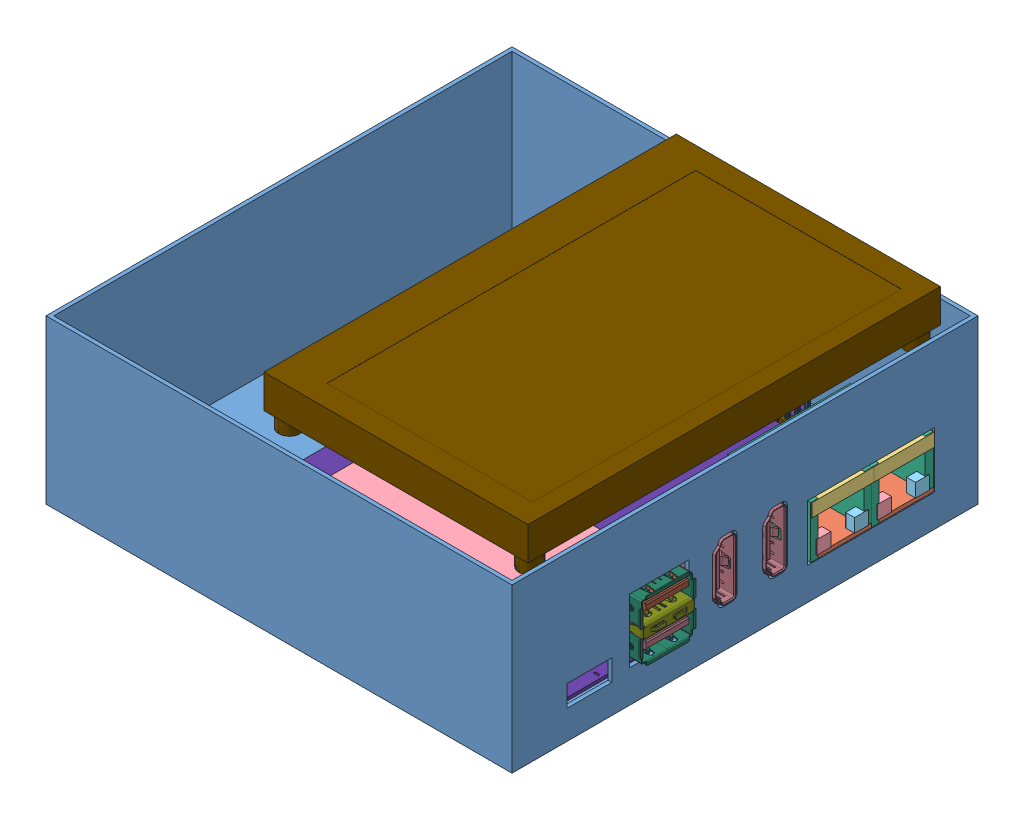
SolidWorks assembly bilbo-hub, configuration Default. Lengths in mm. (continued)
Components (placement in the parent): (continued)
- CM4-DUAL-ETH-4G 5G-BASE-1: CM4-DUAL-ETH-4G 5G-BASE [Default] at (-27.9996 8.7984 -51.6437) x (1 0 0.000117) z (0 1 0) size (91.94 99.62 20.53) (continued)
  - CM4-DUAL-ETH-4G 5G-BASE.step-1: CM4-DUAL-ETH-4G 5G-BASE.step [Default] at origin size (91.94 99.62 20.53) (continued)
    - C49.step-1: C49.step [Default] at origin size (0.8 1.6 0.6) (continued)
      - CAPC1608(0603).step-1: CAPC1608(0603).step [Default] at (38.0407 -61.99 0) x (0 -1 0) z (0 0 1) size (1.6 0.8 0.6)
    - C48.step-1: C48.step [Default] at origin size (1.6 0.8 0.6)
      - CAPC1608(0603).step-1: CAPC1608(0603).step [Default] at (49.0658 -69.8064 0) x (-1 0 0) z (0 0 1) size (1.6 0.8 0.6)
    - C47.step-1: C47.step [Default] at origin size (0.8 1.6 0.6)
      - CAPC1608(0603).step-1: CAPC1608(0603).step [Default] at (39.4963 -61.99 0) x (0 -1 0) z (0 0 1) size (1.6 0.8 0.6)
    - C46.step-1: C46.step [Default] at origin size (1.6 0.8 0.6)
      - CAPC1608(0603).step-1: CAPC1608(0603).step [Default] at (49.0658 -71.2537 0) x (-1 0 0) z (0 0 1) size (1.6 0.8 0.6)
    - C44.step-1: C44.step [Default] at origin size (0.8 1.6 0.6)
      - CAPC1608(0603).step-1: CAPC1608(0603).step [Default] at (42.5195 -81.9688 -0.7984) x (0 1 0) z (0 0 -1) size (1.6 0.8 0.6)
    - C43.step-1: C43.step [Default] at origin size (1.6 0.8 0.6)
      - CAPC1608(0603).step-1: CAPC1608(0603).step [Default] at (49.1866 -62.69 0) x (-1 0 0) z (0 0 1) size (1.6 0.8 0.6)
    - C42.step-1: C42.step [Default] at origin size (1.6 0.8 0.6)
      - CAPC1608(0603).step-1: CAPC1608(0603).step [Default] at (49.0658 -74.1482 0) x (-1 0 0) z (0 0 1) size (1.6 0.8 0.6)
    - C41.step-1: C41.step [Default] at origin size (0.8 1.6 0.6)
      - CAPC1608(0603).step-1: CAPC1608(0603).step [Default] at (52.2225 -27.9219 -0.7984) x (0 1 0) z (0 0 -1) size (1.6 0.8 0.6)
    - C40.step-1: C40.step [Default] at origin size (1.6 0.8 0.6)
      - CAPC1608(0603).step-1: CAPC1608(0603).step [Default] at (49.1866 -63.8607 0) x (-1 0 0) z (0 0 1) size (1.6 0.8 0.6)
    - C39.step-1: C39.step [Default] at origin size (1.6 0.8 0.6)
      - CAPC1608(0603).step-1: CAPC1608(0603).step [Default] at (48.9722 -75.5798 0) x (-1 0 0) z (0 0 1) size (1.6 0.8 0.6)
    - C32.step-1: C32.step [Default] at origin size (1.6 0.8 0.6)
      - CAPC1608(0603).step-1: CAPC1608(0603).step [Default] at (51.5062 -32.7167 -0.7984) x (-1 0 0) z (0 0 -1) size (1.6 0.8 0.6)
    - C31.step-1: C31.step [Default] at origin size (0.8 1.6 0.6)
      - CAPC1608(0603).step-1: CAPC1608(0603).step [Default] at (48.8898 -27.9219 -0.7984) x (0 1 0) z (0 0 -1) size (1.6 0.8 0.6)
    - C30.step-1: C30.step [Default] at origin size (0.8 1.6 0.6)
      - CAPC1608(0603).step-1: CAPC1608(0603).step [Default] at (50.6641 -41.4202 -0.7984) x (0 1 0) z (0 0 -1) size (1.6 0.8 0.6)
    - C28.step-1: C28.step [Default] at origin size (0.8 1.6 0.6)
      - CAPC1608(0603).step-1: CAPC1608(0603).step [Default] at (53.758 -41.4202 -0.7984) x (0 1 0) z (0 0 -1) size (1.6 0.8 0.6)
    - C27.step-1: C27.step [Default] at origin size (0.8 1.6 0.6)
      - CAPC1608(0603).step-1: CAPC1608(0603).step [Default] at (52.2222 -41.4202 -0.7984) x (0 1 0) z (0 0 -1) size (1.6 0.8 0.6)
    - C26.step-1: C26.step [Default] at origin size (1.6 0.8 0.6)
      - CAPC1608(0603).step-1: CAPC1608(0603).step [Default] at (51.5325 -31.2588 -0.7984) x (1 0 0) z (0 0 -1) size (1.6 0.8 0.6)
    - C22.step-1: C22.step [Default] at origin size (1.6 0.8 0.6)
      - CAPC1608(0603).step-1: CAPC1608(0603).step [Default] at (51.5318 -35.5502 -0.7984) x (1 0 0) z (0 0 -1) size (1.6 0.8 0.6)
    - C21.step-1: C21.step [Default] at origin size (1.6 0.8 0.6)
      - CAPC1608(0603).step-1: CAPC1608(0603).step [Default] at (51.5318 -38.3867 -0.7984) x (1 0 0) z (0 0 -1) size (1.6 0.8 0.6)
    - C4.step-1: C4.step [Default] at origin size (0.8 1.6 0.6)
      - CAPC1608(0603).step-1: CAPC1608(0603).step [Default] at (56.9561 -77.7112 -0.7984) x (0 -1 0) z (0 0 -1) size (1.6 0.8 0.6)
    - C3.step-1: C3.step [Default] at origin size (1.27 2.72 0.46)
      - 663598576.step-1: 663598576.step [Default] at (56.9823 -82.7935 -1.2584) size (1.27 0.28 0.46)
        - Extruded-45.step-1: Extruded-45.step [Default] at origin size (1.27 0.28 0.46)
      - 663598576.step-2: 663598576.step [Default] at (56.9823 -80.3446 -1.2584) size (1.27 0.28 0.46)
        - Extruded-45.step-1: Extruded-45.step [Default] at origin size (1.27 0.28 0.46)
      - 764368928.step-1: 764368928.step [Default] at (56.9823 -81.6251 -1.2484) size (1.12 2.29 0.42)
        - Extruded-46.step-1: Extruded-46.step [Default] at origin size (1.12 2.29 0.42)
    - AMS-1.step-1: AMS-1.step [Default] at origin size (6.73 3.43 1.02)
      - 880594240.step-1: 880594240.step [Default] at (36.1772 -86.6648 0.254) size (6.73 3.43 1.02)
        - Extruded-47.step-1: Extruded-47.step [Default] at origin size (6.73 3.43 1.02)
    - R11.step-1: R11.step [Default] at origin size (0.8 1.6 0.38)
      - RESC1608(0603).step-1: RESC1608(0603).step [Default] at (64.5833 -30.5497 -0.7984) x (0 -1 0) z (1 0 0) size (1.6 0.38 0.8)
    - U3.step-1: U3.step [Default] at origin size (7.8 5.3 2.16)
      - 1503579216.step-1: 1503579216.step [Default] at (33.3767 -82.4828 -1.0524) size (1.3 0.41 0.25)
        - Extruded-48.step-1: Extruded-48.step [Default] at origin size (1.3 0.41 0.25)
      - 1503579216.step-2: 1503579216.step [Default] at (33.3767 -81.2128 -1.0524) size (1.3 0.41 0.25)
        - Extruded-48.step-1: Extruded-48.step [Default] at origin size (1.3 0.41 0.25)
      - 1503579216.step-3: 1503579216.step [Default] at (33.3767 -79.9428 -1.0524) size (1.3 0.41 0.25)
        - Extruded-48.step-1: Extruded-48.step [Default] at origin size (1.3 0.41 0.25)
      - 1503579216.step-4: 1503579216.step [Default] at (33.3767 -78.6728 -1.0524) size (1.3 0.41 0.25)
        - Extruded-48.step-1: Extruded-48.step [Default] at origin size (1.3 0.41 0.25)
      - 1503579216.step-5: 1503579216.step [Default] at (39.8767 -82.4928 -1.0524) size (1.3 0.41 0.25)
        - Extruded-48.step-1: Extruded-48.step [Default] at origin size (1.3 0.41 0.25)
      - 1503579216.step-6: 1503579216.step [Default] at (39.8767 -81.2228 -1.0524) size (1.3 0.41 0.25)
        - Extruded-48.step-1: Extruded-48.step [Default] at origin size (1.3 0.41 0.25)
      - 1503579216.step-7: 1503579216.step [Default] at (39.8767 -79.9528 -1.0524) size (1.3 0.41 0.25)
        - Extruded-48.step-1: Extruded-48.step [Default] at origin size (1.3 0.41 0.25)
      - 1503579216.step-8: 1503579216.step [Default] at (39.8767 -78.6828 -1.0524) size (1.3 0.41 0.25)
        - Extruded-48.step-1: Extruded-48.step [Default] at origin size (1.3 0.41 0.25)
      - 1503581520.step-1: 1503581520.step [Default] at (36.6267 -80.5828 -2.9584) size (5.4 5.3 2.01)
        - Extruded-49.step-1: Extruded-49.step [Default] at origin size (5.4 5.3 2.01)
    - R18.step-1: R18.step [Default] at origin size (0.8 1.6 0.38)
      - RESC1608(0603).step-1: RESC1608(0603).step [Default] at (36.3808 -80.8002 0) x (0 -1 0) z (-1 0 0) size (1.6 0.38 0.8)
    - R17.step-1: R17.step [Default] at origin size (1.6 0.8 0.38)
      - RESC1608(0603).step-1: RESC1608(0603).step [Default] at (29.8754 -75.3761 0) x (-1 0 0) z (0 1 0) size (1.6 0.38 0.8)
    - R16.step-1: R16.step [Default] at origin size (0.8 1.6 0.38)
      - RESC1608(0603).step-1: RESC1608(0603).step [Default] at (30.3209 -79.2715 -0.7984) x (0 -1 0) z (1 0 0) size (1.6 0.38 0.8)
    - R15.step-1: R15.step [Default] at origin size (0.8 1.6 0.38)
      - RESC1608(0603).step-1: RESC1608(0603).step [Default] at (50.6744 -27.9001 -0.7984) x (0 1 0) z (-1 0 0) size (1.6 0.38 0.8)
    - U4.step-1: U4.step [Default] at origin size (2.7 2.7 0.45)
      - 880596160.step-1: 880596160.step [Default] at (49.7296 -17.227 -1.2984) size (2.7 2.7 0.45)
        - Extruded-50.step-1: Extruded-50.step [Default] at origin size (2.7 2.7 0.45)
    - U5.step-1: U5.step [Default] at origin size (2 2.1 0.95)
      - User_Library-SC70-5-1.step-1: User_Library-SC70-5-1.step [Default] at (52.8539 -17.1936 -0.7984) x (1 0 0) z (0 0 -1) size (2 2.1 0.95)
    - R35.step-1: R35.step [Default] at origin size (0.8 1.6 0.38)
      - RESC1608(0603).step-1: RESC1608(0603).step [Default] at (52.2527 -11.5783 -0.7984) x (0 1 0) z (-1 0 0) size (1.6 0.38 0.8)
    - R33.step-1: R33.step [Default] at origin size (0.8 1.6 0.38)
      - RESC1608(0603).step-1: RESC1608(0603).step [Default] at (53.7884 -11.5783 -0.7984) x (0 1 0) z (-1 0 0) size (1.6 0.38 0.8)
    - D6.step-1: D6.step [Default] at origin size (1.35 2.6 1.14)
      - SW3dPS-SOD-323.step-1: SW3dPS-SOD-323.step [Default] at (51.0946 -21.502 -0.7984) x (0 -1 0) z (0 0 -1) size (2.6 1.35 1.14)
    - D5.step-1: D5.step [Default] at origin size (1.35 2.6 1.14)
      - SW3dPS-SOD-323.step-1: SW3dPS-SOD-323.step [Default] at (53.3476 -21.502 -0.7984) x (0 -1 0) z (0 0 -1) size (2.6 1.35 1.14)
    - C134.step-1: C134.step [Default] at origin size (0.8 1.6 0.6)
      - CAPC1608(0603).step-1: CAPC1608(0603).step [Default] at (55.1652 -21.3602 -0.7984) x (0 1 0) z (0 0 -1) size (1.6 0.8 0.6)
    - C133.step-1: C133.step [Default] at origin size (0.8 1.6 0.6)
      - CAPC1608(0603).step-1: CAPC1608(0603).step [Default] at (49.1745 -21.3865 -0.7984) x (0 -1 0) z (0 0 -1) size (1.6 0.8 0.6)
    - C38.step-1: C38.step [Default] at origin size (1.6 0.8 0.6)
      - CAPC1608(0603).step-1: CAPC1608(0603).step [Default] at (54.6319 -14.1546 -0.7984) x (1 0 0) z (0 0 -1) size (1.6 0.8 0.6)
    - C37.step-1: C37.step [Default] at origin size (0.8 1.6 0.6)
      - CAPC1608(0603).step-1: CAPC1608(0603).step [Default] at (55.1653 -17.2646 -0.7984) x (0 1 0) z (0 0 -1) size (1.6 0.8 0.6)
    - C36.step-1: C36.step [Default] at origin size (0.8 1.6 0.6)
      - CAPC1608(0603).step-1: CAPC1608(0603).step [Default] at (50.7103 -11.6263 -0.7984) x (0 -1 0) z (0 0 -1) size (1.6 0.8 0.6)
    - C35.step-1: C35.step [Default] at origin size (0.8 1.6 0.6)
      - CAPC1608(0603).step-1: CAPC1608(0603).step [Default] at (49.1745 -11.6263 -0.7984) x (0 -1 0) z (0 0 -1) size (1.6 0.8 0.6)
    - C9.step-1: C9.step [Default] at origin size (0.8 1.6 0.6)
      - CAPC1608(0603).step-1: CAPC1608(0603).step [Default] at (17.7596 -11.9503 -0.7984) x (0 1 0) z (0 0 -1) size (1.6 0.8 0.6)
    - C14.step-1: C14.step [Default] at origin size (0.8 1.6 0.6)
      - CAPC1608(0603).step-1: CAPC1608(0603).step [Default] at (77.2667 -94.9453 -0.7984) x (0 -1 0) z (0 0 -1) size (1.6 0.8 0.6)
    - C1.step-1: C1.step [Default] at origin size (0.8 1.6 0.6)
      - CAPC1608(0603).step-1: CAPC1608(0603).step [Default] at (39.7941 -94.4916 -0.7984) x (0 -1 0) z (0 0 -1) size (1.6 0.8 0.6)
    - U15.step-1: U15.step [Default] at origin size (2.5 3 1.1)
      - SW3DPS-SOT-23-5-DEFAULT.step-1: SW3DPS-SOT-23-5-DEFAULT.step [Default] at (9.4742 -18.2293 -1.2984) x (0 1 0) z (-1 0 0) size (3 1.1 2.5)
    - U12.step-1: U12.step [Default] at origin size (1.01 2.5 0.55)
      - User_Library-UDFN10.step-1: User_Library-UDFN10.step [Default] at (62.7073 -10.1236 0.1516) x (0 -1 0) z (1 0 0) size (2.5 0.55 1.01)
        - Body.step-1: Body.step [Default] at (1.0785 0.9721 1.8983) size (2.5 0.5 1)
        - Pin1.step-1: Pin1.step [Default] at (0.0785 1.0521 2.2208) x (0 0 -1) z (-1 0 0) size (0.36 0.13 0.2)
        - Pin2.step-1: Pin2.step [Default] at (0.5785 1.0521 2.2208) x (0 0 1) z (1 0 0) size (0.36 0.13 0.2)
        - Pin4.step-1: Pin4.step [Default] at (1.0785 0.9221 2.2208) x (0 0 1) z (-1 0 0) size (0.49 0.13 0.4)
        - Pin2.step-2: Pin2.step [Default] at (1.5785 0.9221 2.2208) x (0 0 1) z (-1 0 0) size (0.36 0.13 0.2)
        - Pin2.step-3: Pin2.step [Default] at (2.0785 0.9221 2.2208) x (0 0 1) z (-1 0 0) size (0.36 0.13 0.2)
        - Pin2.step-4: Pin2.step [Default] at (2.0785 0.9221 1.5758) x (0 0 -1) z (1 0 0) size (0.36 0.13 0.2)
        - Pin2.step-5: Pin2.step [Default] at (1.5785 0.9221 1.5758) x (0 0 -1) z (1 0 0) size (0.36 0.13 0.2)
        - Pin3.step-1: Pin3.step [Default] at (1.0785 0.9221 1.5758) x (0 0 1) z (-1 0 0) size (0.36 0.13 0.4)
        - Pin2.step-6: Pin2.step [Default] at (0.5785 0.9221 1.5758) x (0 0 -1) z (1 0 0) size (0.36 0.13 0.2)
        - Pin2.step-7: Pin2.step [Default] at (0.0785 0.9221 1.5758) x (0 0 -1) z (1 0 0) size (0.36 0.13 0.2)
    - U11.step-1: U11.step [Default] at origin size (2.5 3 1.1)
      - SW3DPS-SOT-23-5-DEFAULT.step-1: SW3DPS-SOT-23-5-DEFAULT.step [Default] at (50.4006 -45.1237 -1.2984) x (0 -1 0) z (1 0 0) size (3 1.1 2.5)
    - U9.step-1: U9.step [Default] at origin size (1.01 2.5 0.55)
      - User_Library-UDFN10.step-1: User_Library-UDFN10.step [Default] at (66.4724 -18.6329 0.1516) x (0 1 0) z (-1 0 0) size (2.5 0.55 1.01)
        - Body.step-1: Body.step [Default] at (1.0785 0.9721 1.8983) size (2.5 0.5 1)
        - Pin1.step-1: Pin1.step [Default] at (0.0785 1.0521 2.2208) x (0 0 -1) z (-1 0 0) size (0.36 0.13 0.2)
        - Pin2.step-1: Pin2.step [Default] at (0.5785 1.0521 2.2208) x (0 0 1) z (1 0 0) size (0.36 0.13 0.2)
        - Pin4.step-1: Pin4.step [Default] at (1.0785 0.9221 2.2208) x (0 0 1) z (-1 0 0) size (0.49 0.13 0.4)
        - Pin2.step-2: Pin2.step [Default] at (1.5785 0.9221 2.2208) x (0 0 1) z (-1 0 0) size (0.36 0.13 0.2)
        - Pin2.step-3: Pin2.step [Default] at (2.0785 0.9221 2.2208) x (0 0 1) z (-1 0 0) size (0.36 0.13 0.2)
        - Pin2.step-4: Pin2.step [Default] at (2.0785 0.9221 1.5758) x (0 0 -1) z (1 0 0) size (0.36 0.13 0.2)
        - Pin2.step-5: Pin2.step [Default] at (1.5785 0.9221 1.5758) x (0 0 -1) z (1 0 0) size (0.36 0.13 0.2)
        - Pin3.step-1: Pin3.step [Default] at (1.0785 0.9221 1.5758) x (0 0 1) z (-1 0 0) size (0.36 0.13 0.4)
        - Pin2.step-6: Pin2.step [Default] at (0.5785 0.9221 1.5758) x (0 0 -1) z (1 0 0) size (0.36 0.13 0.2)
        - Pin2.step-7: Pin2.step [Default] at (0.0785 0.9221 1.5758) x (0 0 -1) z (1 0 0) size (0.36 0.13 0.2)
    - R64.step-1: R64.step [Default] at origin size (0.8 1.6 0.38)
      - RESC1608(0603).step-1: RESC1608(0603).step [Default] at (12.5285 -18.2821 -0.7984) x (0 -1 0) z (1 0 0) size (1.6 0.38 0.8)
    - R57.step-1: R57.step [Default] at origin size (1.6 0.8 0.38)
      - RESC1608(0603).step-1: RESC1608(0603).step [Default] at (10.7955 -85.6126 0) x (-1 0 0) z (0 1 0) size (1.6 0.38 0.8)
    - R56.step-1: R56.step [Default] at origin size (1.6 0.8 0.38)
      - RESC1608(0603).step-1: RESC1608(0603).step [Default] at (10.8653 -83.8424 0) x (1 0 0) z (0 -1 0) size (1.6 0.38 0.8)
    - R55.step-1: R55.step [Default] at origin size (0.8 1.6 0.38)
      - RESC1608(0603).step-1: RESC1608(0603).step [Default] at (15.5482 -18.2821 -0.7984) x (0 -1 0) z (1 0 0) size (1.6 0.38 0.8)
    - R47.step-1: R47.step [Default] at origin size (0.8 1.6 0.38)
      - RESC1608(0603).step-1: RESC1608(0603).step [Default] at (55.3094 -11.6398 -0.7984) x (0 -1 0) z (1 0 0) size (1.6 0.38 0.8)
    - R46.step-1: R46.step [Default] at origin size (0.8 1.6 0.38)
      - RESC1608(0603).step-1: RESC1608(0603).step [Default] at (64.5833 -21.1257 -0.7984) x (0 -1 0) z (1 0 0) size (1.6 0.38 0.8)
    - R44.step-1: R44.step [Default] at origin size (0.8 1.6 0.38)
      - RESC1608(0603).step-1: RESC1608(0603).step [Default] at (19.5056 -11.9983 -0.7984) x (0 -1 0) z (1 0 0) size (1.6 0.38 0.8)
    - C84.step-1: C84.step [Default] at origin size (0.8 1.6 0.6)
      - CAPC1608(0603).step-1: CAPC1608(0603).step [Default] at (53.3602 -45.0643 -0.7984) x (0 -1 0) z (0 0 -1) size (1.6 0.8 0.6)
    - C83.step-1: C83.step [Default] at origin size (0.8 1.6 0.6)
      - CAPC1608(0603).step-1: CAPC1608(0603).step [Default] at (48.8898 -41.5988 -0.7984) x (0 -1 0) z (0 0 -1) size (1.6 0.8 0.6)
    - C82.step-1: C82.step [Default] at origin size (0.8 1.6 0.6)
      - CAPC1608(0603).step-1: CAPC1608(0603).step [Default] at (5.0212 -18.2595 -0.7984) x (0 -1 0) z (0 0 -1) size (1.6 0.8 0.6)
    - C79.step-1: C79.step [Default] at origin size (0.8 1.6 0.6)
      - CAPC1608(0603).step-1: CAPC1608(0603).step [Default] at (64.5899 -14.3235 -0.7984) x (0 1 0) z (0 0 -1) size (1.6 0.8 0.6)
    - C75.step-1: C75.step [Default] at origin size (0.8 1.6 0.6)
      - CAPC1608(0603).step-1: CAPC1608(0603).step [Default] at (6.5827 -18.234 -0.7984) x (0 1 0) z (0 0 -1) size (1.6 0.8 0.6)
    - C74.step-1: C74.step [Default] at origin size (0.8 1.6 0.6)
      - CAPC1608(0603).step-1: CAPC1608(0603).step [Default] at (14.0516 -18.2603 -0.7984) x (0 -1 0) z (0 0 -1) size (1.6 0.8 0.6)
    - C10.step-1: C10.step [Default] at origin size (0.8 1.6 0.6)
      - CAPC1608(0603).step-1: CAPC1608(0603).step [Default] at (50.1741 -81.8813 -0.7984) x (0 -1 0) z (0 0 -1) size (1.6 0.8 0.6)
    - C11.step-1: C11.step [Default] at origin size (0.8 1.6 0.6)
      - CAPC1608(0603).step-1: CAPC1608(0603).step [Default] at (48.3709 -81.855 -0.7984) x (0 1 0) z (0 0 -1) size (1.6 0.8 0.6)
    - C15.step-1: C15.step [Default] at origin size (0.8 1.6 0.6)
      - CAPC1608(0603).step-1: CAPC1608(0603).step [Default] at (59.8371 -27.9482 -0.7984) x (0 -1 0) z (0 0 -1) size (1.6 0.8 0.6)
    - C16.step-1: C16.step [Default] at origin size (1.6 0.8 0.6)
      - CAPC1608(0603).step-1: CAPC1608(0603).step [Default] at (51.5318 -36.9668 -0.7984) x (1 0 0) z (0 0 -1) size (1.6 0.8 0.6)
    - R8.step-1: R8.step [Default] at origin size (1.6 0.8 0.38)
      - RESC1608(0603).step-1: RESC1608(0603).step [Default] at (29.9452 -70.3512 0) x (1 0 0) z (0 -1 0) size (1.6 0.38 0.8)
    - R10.step-1: R10.step [Default] at origin size (0.8 1.6 0.38)
      - RESC1608(0603).step-1: RESC1608(0603).step [Default] at (42.5007 -79.0493 -0.7984) x (0 1 0) z (-1 0 0) size (1.6 0.38 0.8)
    - R12.step-1: R12.step [Default] at origin size (0.8 1.6 0.38)
      - RESC1608(0603).step-1: RESC1608(0603).step [Default] at (64.5936 -24.0283 -0.7984) x (0 1 0) z (-1 0 0) size (1.6 0.38 0.8)
    - U1.step-1: U1.step [Default] at origin size (2.5 3 1.1)
      - SW3DPS-SOT-23-5-DEFAULT.step-1: SW3DPS-SOT-23-5-DEFAULT.step [Default] at (53.5777 -77.8952 -1.2984) x (0 -1 0) z (1 0 0) size (3 1.1 2.5)
    - C19.step-1: C19.step [Default] at origin size (0.8 1.6 0.6)
      - CAPC1608(0603).step-1: CAPC1608(0603).step [Default] at (61.4628 -41.4202 -0.7984) x (0 1 0) z (0 0 -1) size (1.6 0.8 0.6)
    - TF1.step-1: TF1.step [Default] at origin size (13.82 14.45 2.1)
      - 1103521424.step-1: 1103521424.step [Default] at (7.383 -29.5195 -2.8984) size (13.82 14.45 0.1)
        - Extruded-51.step-1: Extruded-51.step [Default] at origin size (13.82 14.45 0.1)
      - 1103521296.step-1: 1103521296.step [Default] at (7.383 -29.5195 -2.8984) size (13.82 14.45 2.1)
        - Extruded-52.step-1: Extruded-52.step [Default] at origin size (13.82 14.45 2.1)
      - 1103521168.step-1: 1103521168.step [Default] at (7.383 -29.5195 -1.2984) size (13.82 14.45 0.5)
        - Extruded-53.step-1: Extruded-53.step [Default] at origin size (13.82 14.45 0.5)
    - CM-R1.step-1: CM-R1.step [Default] at origin size (0.85 1.65 0.46)
      - 575262224.step-1: 575262224.step [Default] at (42.7492 -93.7926 -1.2584) size (0.85 0.28 0.46)
        - Extruded-54.step-1: Extruded-54.step [Default] at origin size (0.85 0.28 0.46)
      - 575262224.step-2: 575262224.step [Default] at (42.7492 -95.1642 -1.2584) size (0.85 0.28 0.46)
        - Extruded-54.step-1: Extruded-54.step [Default] at origin size (0.85 0.28 0.46)
      - 575262352.step-1: 575262352.step [Default] at (42.7492 -94.4784 -1.2484) size (0.8 1.5 0.42)
        - Extruded-55.step-1: Extruded-55.step [Default] at origin size (0.8 1.5 0.42)
    - CM-R4.step-1: CM-R4.step [Default] at origin size (0.85 1.65 0.46)
      - 575262224.step-1: 575262224.step [Default] at (41.2717 -93.7926 -1.2584) size (0.85 0.28 0.46)
        - Extruded-54.step-1: Extruded-54.step [Default] at origin size (0.85 0.28 0.46)
      - 575262224.step-2: 575262224.step [Default] at (41.2717 -95.1642 -1.2584) size (0.85 0.28 0.46)
        - Extruded-54.step-1: Extruded-54.step [Default] at origin size (0.85 0.28 0.46)
      - 575262352.step-1: 575262352.step [Default] at (41.2717 -94.4784 -1.2484) size (0.8 1.5 0.42)
        - Extruded-55.step-1: Extruded-55.step [Default] at origin size (0.8 1.5 0.42)
    - L1.step-1: L1.step [Default] at origin size (9.95 4.45 11.5)
      - 1015527952.step-1: 1015527952.step [Default] at (7.7605 -62.6584 -1.5) x (0 1 0) z (0 0 1) size (0.76 0.76 5)
        - Cylinder.step-1: Cylinder.step [Default] at origin size (0.76 0.76 5)
      - 1015527952.step-2: 1015527952.step [Default] at (5.2205 -62.6584 -1.5) x (0 1 0) z (0 0 1) size (0.76 0.76 5)
        - Cylinder.step-1: Cylinder.step [Default] at origin size (0.76 0.76 5)
      - 1015527952.step-3: 1015527952.step [Default] at (5.2205 -60.1183 -1.5) x (0 1 0) z (0 0 1) size (0.76 0.76 5)
        - Cylinder.step-1: Cylinder.step [Default] at origin size (0.76 0.76 5)
      - 1015527952.step-4: 1015527952.step [Default] at (7.7605 -60.1183 -1.5) x (0 1 0) z (0 0 1) size (0.76 0.76 5)
        - Cylinder.step-1: Cylinder.step [Default] at origin size (0.76 0.76 5)
      - 1015527832.step-1: 1015527832.step [Default] at (0.9405 -61.3885 8) x (0 -1 0) z (0 0 1) size (3.5 3.5 3.5)
        - Sphere-13.step-1: Sphere-13.step [Default] at origin size (3.5 3.5 3.5)
      - 1103520528.step-1: 1103520528.step [Default] at (4.6411 -61.3877 0.254) size (9 4.45 9.75)
        - Extruded-12.step-1: Extruded-12.step [Default] at origin size (9 4.45 9.75)
      - 1015527712.step-1: 1015527712.step [Default] at (0.9405 -61.3885 3) x (0 -1 0) z (0 0 1) size (3.5 3.5 3.5)
        - Sphere.step-1: Sphere.step [Default] at origin size (3.5 3.5 3.5)
    - C45.step-1: C45.step [Default] at origin size (0.8 1.6 0.6)
      - CAPC1608(0603).step-1: CAPC1608(0603).step [Default] at (58.2116 -27.9482 -0.7984) x (0 -1 0) z (0 0 -1) size (1.6 0.8 0.6)
    - C12.step-1: C12.step [Default] at origin size (1.6 0.8 0.6)
      - CAPC1608(0603).step-1: CAPC1608(0603).step [Default] at (11.4515 -63.7998 -0.7984) x (1 0 0) z (0 0 -1) size (1.6 0.8 0.6)
    - C13.step-1: C13.step [Default] at origin size (1.6 0.8 0.6)
      - CAPC1608(0603).step-1: CAPC1608(0603).step [Default] at (16.0523 -67.4574 -0.7984) x (-1 0 0) z (0 0 -1) size (1.6 0.8 0.6)
    - Q5.step-1: Q5.step [Default] at origin size (2.64 3 1.08)
      - ALSRobot-SOT23.step-1: ALSRobot-SOT23.step [Default] at (17.3302 -60.1735 -0.7984) x (0 -1 0) z (0 0 -1) size (3 2.64 1.08)
    - R21.step-1: R21.step [Default] at origin size (1.6 0.8 0.38)
      - RESC1608(0603).step-1: RESC1608(0603).step [Default] at (11.4034 -65.5434 -0.7984) x (-1 0 0) z (0 -1 0) size (1.6 0.38 0.8)
    - R45.step-1: R45.step [Default] at origin size (1.6 0.8 0.38)
      - RESC1608(0603).step-1: RESC1608(0603).step [Default] at (20.7078 -63.8076 -0.7984) x (-1 0 0) z (0 -1 0) size (1.6 0.38 0.8)
    - R48.step-1: R48.step [Default] at origin size (1.6 3.2 0.6)
      - User_Library-CR3216-1206.step-1: User_Library-CR3216-1206.step [Default] at (21.1402 -59.9705 -0.7984) x (0 -1 0) z (1 0 0) size (3.2 0.6 1.6)
    - R49.step-1: R49.step [Default] at origin size (1.6 0.8 0.38)
      - RESC1608(0603).step-1: RESC1608(0603).step [Default] at (20.7776 -67.2557 -0.7984) x (1 0 0) z (0 1 0) size (1.6 0.38 0.8)
    - U2.step-1: U2.step [Default] at origin size (1.19 2.9 1.14)
      - 880594496.step-1: 880594496.step [Default] at (16.073 -64.5424 -1.9414) size (1.19 2.9 1.14)
        - Extruded-56.step-1: Extruded-56.step [Default] at origin size (1.19 2.9 1.14)
    - R74.step-1: R74.step [Default] at origin size (1.6 0.8 0.38)
      - RESC1608(0603).step-1: RESC1608(0603).step [Default] at (84.1244 -89.9694 -0.7984) x (1 0 0) z (0 1 0) size (1.6 0.38 0.8)
    - R75.step-1: R75.step [Default] at origin size (1.6 0.8 0.38)
      - RESC1608(0603).step-1: RESC1608(0603).step [Default] at (84.1244 -92.9694 -0.7984) x (1 0 0) z (0 1 0) size (1.6 0.38 0.8)
    - C103.step-1: C103.step [Default] at origin size (0.8 1.6 0.6)
      - CAPC1608(0603).step-1: CAPC1608(0603).step [Default] at (63.7716 -88.7373 -0.7984) x (0 -1 0) z (0 0 -1) size (1.6 0.8 0.6)
    - C104.step-1: C104.step [Default] at origin size (0.85 1.65 0.46)
      - 575262352.step-1: 575262352.step [Default] at (77.2669 -91.76 -1.2484) size (0.8 1.5 0.42)
        - Extruded-55.step-1: Extruded-55.step [Default] at origin size (0.8 1.5 0.42)
      - 575262224.step-1: 575262224.step [Default] at (77.2669 -92.4458 -1.2584) size (0.85 0.28 0.46)
        - Extruded-54.step-1: Extruded-54.step [Default] at origin size (0.85 0.28 0.46)
      - 575262224.step-2: 575262224.step [Default] at (77.2669 -91.0743 -1.2584) size (0.85 0.28 0.46)
        - Extruded-54.step-1: Extruded-54.step [Default] at origin size (0.85 0.28 0.46)
    - C105.step-1: C105.step [Default] at origin size (1.6 0.8 0.6)
      - CAPC1608(0603).step-1: CAPC1608(0603).step [Default] at (63.0809 -82.1182 -0.7984) x (-1 0 0) z (0 0 -1) size (1.6 0.8 0.6)
    - C106.step-1: C106.step [Default] at origin size (1.6 0.8 0.6)
      - CAPC1608(0603).step-1: CAPC1608(0603).step [Default] at (59.2175 -84.7976 -0.7984) x (1 0 0) z (0 0 -1) size (1.6 0.8 0.6)
    - C107.step-1: C107.step [Default] at origin size (1.65 0.85 0.46)
      - 575261968.step-1: 575261968.step [Default] at (68.0384 -80.896 -1.2484) size (1.5 0.8 0.42)
        - Extruded-4.step-1: Extruded-4.step [Default] at origin size (1.5 0.8 0.42)
      - 575262096.step-1: 575262096.step [Default] at (68.7242 -80.896 -1.2584) size (0.28 0.85 0.46)
        - Extruded-5.step-1: Extruded-5.step [Default] at origin size (0.28 0.85 0.46)
      - 575262096.step-2: 575262096.step [Default] at (67.3526 -80.896 -1.2584) size (0.28 0.85 0.46)
        - Extruded-5.step-1: Extruded-5.step [Default] at origin size (0.28 0.85 0.46)
    - C108.step-1: C108.step [Default] at origin size (1.6 0.8 0.6)
      - CAPC1608(0603).step-1: CAPC1608(0603).step [Default] at (68.0257 -79.3085 -0.7984) x (-1 0 0) z (0 0 -1) size (1.6 0.8 0.6)
    - R76.step-1: R76.step [Default] at origin size (0.8 1.6 0.38)
      - RESC1608(0603).step-1: RESC1608(0603).step [Default] at (61.9749 -88.6896 -0.7984) x (0 1 0) z (-1 0 0) size (1.6 0.38 0.8)
    - R77.step-1: R77.step [Default] at origin size (1.6 0.8 0.38)
      - RESC1608(0603).step-1: RESC1608(0603).step [Default] at (59.1749 -86.3098 -0.7984) x (-1 0 0) z (0 -1 0) size (1.6 0.38 0.8)
    - R79.step-1: R79.step [Default] at origin size (1.6 0.8 0.38)
      - RESC1608(0603).step-1: RESC1608(0603).step [Default] at (59.1749 -87.8287 -0.7984) x (-1 0 0) z (0 -1 0) size (1.6 0.38 0.8)
    - R80.step-1: R80.step [Default] at origin size (1.6 0.8 0.38)
      - RESC1608(0603).step-1: RESC1608(0603).step [Default] at (59.2447 -89.3608 -0.7984) x (1 0 0) z (0 1 0) size (1.6 0.38 0.8)
    - U16.step-1: U16.step [Default] at origin size (1.81 1.7 0.55)
      - 661965792.step-1: 661965792.step [Default] at (62.1545 -85.5846 -0.9584) size (0.4 0.23 0.16)
        - Extruded-57.step-1: Extruded-57.step [Default] at origin size (0.4 0.23 0.16)
      - 661965792.step-2: 661965792.step [Default] at (62.1545 -86.0845 -0.9584) size (0.4 0.23 0.16)
        - Extruded-57.step-1: Extruded-57.step [Default] at origin size (0.4 0.23 0.16)
      - 661965792.step-3: 661965792.step [Default] at (62.1545 -86.5845 -0.9584) size (0.4 0.23 0.16)
        - Extruded-57.step-1: Extruded-57.step [Default] at origin size (0.4 0.23 0.16)
      - 661965792.step-4: 661965792.step [Default] at (63.5565 -86.5846 -0.9584) size (0.4 0.23 0.16)
        - Extruded-57.step-1: Extruded-57.step [Default] at origin size (0.4 0.23 0.16)
      - 661965792.step-5: 661965792.step [Default] at (63.5565 -86.0846 -0.9584) size (0.4 0.23 0.16)
        - Extruded-57.step-1: Extruded-57.step [Default] at origin size (0.4 0.23 0.16)
      - 661965792.step-6: 661965792.step [Default] at (63.5565 -85.5846 -0.9584) size (0.4 0.23 0.16)
        - Extruded-57.step-1: Extruded-57.step [Default] at origin size (0.4 0.23 0.16)
      - 1348844112.step-1: 1348844112.step [Default] at (62.8544 -86.0846 -1.3484) size (1.3 1.7 0.5)
        - Extruded-58.step-1: Extruded-58.step [Default] at origin size (1.3 1.7 0.5)
    - C93.step-1: C93.step [Default] at origin size (1.6 0.8 0.6)
      - CAPC1608(0603).step-1: CAPC1608(0603).step [Default] at (14.7077 -83.849 0) x (1 0 0) z (0 0 1) size (1.6 0.8 0.6)
    - R6.step-1: R6.step [Default] at origin size (3.44 1.51 0.46)
      - 575262608.step-1: 575262608.step [Default] at (65.5642 -79.6989 -1.2584) size (0.28 1.51 0.46)
        - Extruded-59.step-1: Extruded-59.step [Default] at origin size (0.28 1.51 0.46)
      - 575262608.step-2: 575262608.step [Default] at (62.4017 -79.699 -1.2584) size (0.28 1.51 0.46)
        - Extruded-59.step-1: Extruded-59.step [Default] at origin size (0.28 1.51 0.46)
      - 1127966432.step-1: 1127966432.step [Default] at (63.9893 -79.7069 -1.2484) size (3.05 1.38 0.42)
        - Extruded-60.step-1: Extruded-60.step [Default] at origin size (3.05 1.38 0.42)
    - C87.step-1: C87.step [Default] at origin size (1.65 0.85 0.46)
      - 575261968.step-1: 575261968.step [Default] at (66.2355 -91.4092 -1.2484) size (1.5 0.8 0.42)
        - Extruded-4.step-1: Extruded-4.step [Default] at origin size (1.5 0.8 0.42)
      - 575262096.step-1: 575262096.step [Default] at (65.5498 -91.4092 -1.2584) size (0.28 0.85 0.46)
        - Extruded-5.step-1: Extruded-5.step [Default] at origin size (0.28 0.85 0.46)
      - 575262096.step-2: 575262096.step [Default] at (66.9213 -91.4092 -1.2584) size (0.28 0.85 0.46)
        - Extruded-5.step-1: Extruded-5.step [Default] at origin size (0.28 0.85 0.46)
    - U10.step-1: U10.step [Default] at origin size (4.94 3.1 1.1)
      - User_Library-MSOP8.step-1: User_Library-MSOP8.step [Default] at (68.0617 -93.7668 -1.8984) x (1 0 0) z (0 1 0) size (4.94 1.1 3.1)
    - C20.step-1: C20.step [Default] at origin size (1.6 0.8 0.6)
      - CAPC1608(0603).step-1: CAPC1608(0603).step [Default] at (11.4514 -67.2408 -0.7984) x (1 0 0) z (0 0 -1) size (1.6 0.8 0.6)
    - HDMI0.step-1: HDMI0.step [Default] at origin size (23.1 7.88 20.15)
      - 72r3759_2007435-1.step-1: 72r3759_2007435-1.step [Default] at (88.2992 -56.8507 9) x (0 1 0) z (1 0 0) size (7.88 20.15 23.1)
    - Board.step-1: Board.step [Default] at (0 0 -0.7984) size (87.02 99.62 0.8)
- screen-1: screen [Default] at (23 47.0396 -0.2185) x (0 0 1) z (0 -1 0) size (106.2 68 14)
Mates (geometry in assembly coordinates):
- Distance1: distance = 6 mm anti-aligned: plane of box_lower-1 through (0 2 0) normal (0 1 0); plane of CM4-DUAL-ETH-4G 5G-BASE-1/CM4-DUAL-ETH-4G 5G-BASE.step-1/Board.step-1 through (-27.9785 8 45.0055) normal (0 -1 0)
- Distance2: distance = 1 mm aligned: plane of box_lower-1 through (60 2 60) normal (1 0 0); plane of CM4-DUAL-ETH-4G 5G-BASE-1/CM4-DUAL-ETH-4G 5G-BASE.step-1/Board.step-1 through (59 8 44.4664) normal (1 0 0)
- Parallel4: parallel anti-aligned: plane of box_lower-1 through (0 2 0) normal (0 1 0); plane of screen-1 through (-19.9235 41.7896 63.6957) normal (0 -1 0)
- Parallel5: parallel anti-aligned: plane of box_lower-1 through (-59 42 -59) normal (1 0 0); plane of screen-1 through (-11 62.0396 52.8815) normal (-1 0 0)
- Distance4: distance = 2 mm anti-aligned: plane of screen-1 through (57 62.0396 -53.3185) normal (1 0 0); plane of box_lower-1 through (59 42 -59) normal (-1 0 0)
